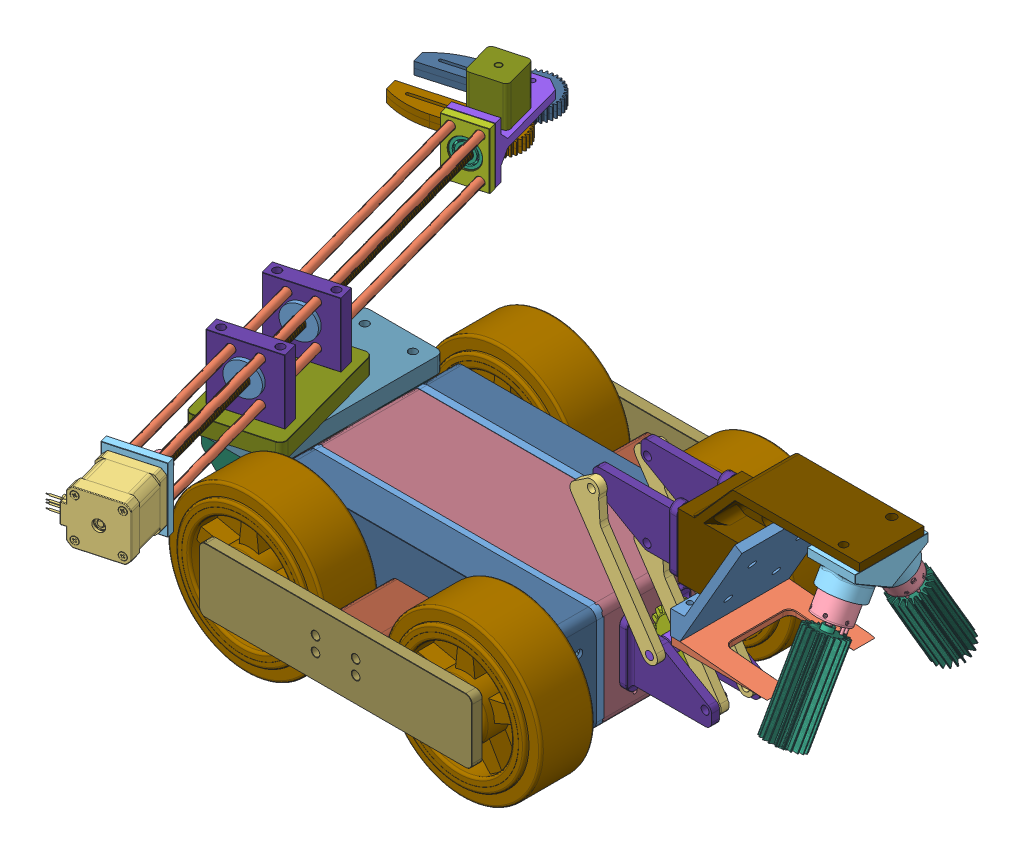
SolidWorks assembly __FINAL_DESIGN, configuration Default. Lengths in mm.
Overall size (608.35 222.7 508.61).
168 component instances, 44 part files, 1 mates.
Components (placement in the parent):
- Chassis-1: Chassis [Default] at origin size (228.6 82.55 202.26)
  - WheelAssy-1: WheelAssy [Default] at origin size (228.6 82.55 139.03)
    - ChassisSidePlate-1: ChassisSidePlate [Default] at origin size (228.6 82.55 6.35)
    - DriveStepper-2: DriveStepper [Default] at (-33.528 0 6.35) x (0 1 0) z (0 0 -1) size (56.9 64.15 97)
    - 60355K503_BALL BEARING-1: 60355K503_BALL BEARING [60355K503] at (85.598 0 1.905) x (-0.923728 -0.383049 0) z (0 0 1) size (15.88 15.88 4.76)
    - 1327K113_MINIATURE 12L14 DRIVE STEEL SHAFT-1: 1327K113_MINIATURE 12L14 DRIVE STEEL SHAFT [1327K113] at (85.598 0 -18.5798) x (-0.959536 -0.281585 0) z (0 0 1) size (6.35 6.35 76.2)
    - 60355K503_BALL BEARING-2: 60355K503_BALL BEARING [60355K503] at (-85.598 0 2.0926) size (15.88 15.88 4.76)
    - 1327K113_MINIATURE 12L14 DRIVE STEEL SHAFT-2: 1327K113_MINIATURE 12L14 DRIVE STEEL SHAFT [1327K113] at (-85.598 0 -16.8162) x (-0.027859 0.999612 0) z (0 0 1) size (6.35 6.35 76.2)
    - 2737T131_FINISHED-BORE SPROCKET FOR ANSI ROLLER CHAIN-1: 2737T131_FINISHED-BORE SPROCKET FOR ANSI ROLLER CHAIN [2737T131] at (85.598 0 -14.478) x (0.999569 0.029358 0) z (0 0 1) size (43.9 43.9 15.88)
    - 2737T131_FINISHED-BORE SPROCKET FOR ANSI ROLLER CHAIN-2: 2737T131_FINISHED-BORE SPROCKET FOR ANSI ROLLER CHAIN [2737T131] at (-85.598 0 -14.478) x (0.999569 0.029358 0) z (0 0 1) size (43.9 43.9 15.88)
    - 6261K281_ROLLER CHAIN-1: 6261K281_ROLLER CHAIN [6261K281] at (-14.2774 -20.8743 -13.97) x (-0.999974 0.007172 0) z (0 0 1) size (18.33 5.99 7.62)
    - 6261K281_ROLLER CHAIN-2: 6261K281_ROLLER CHAIN [6261K281] at (-26.9771 -20.7832 -13.97) x (-0.999974 0.007172 0) z (0 0 1) size (18.33 5.99 7.62)
    - 6261K281_ROLLER CHAIN-3: 6261K281_ROLLER CHAIN [6261K281] at (-39.6768 -20.6921 -13.97) x (-0.999974 0.007172 0) z (0 0 1) size (18.33 5.99 7.62)
    - 6261K281_ROLLER CHAIN-4: 6261K281_ROLLER CHAIN [6261K281] at (-52.3765 -20.601 -13.97) x (-0.999974 0.007172 0) z (0 0 1) size (18.33 5.99 7.62)
    - 6261K281_ROLLER CHAIN-5: 6261K281_ROLLER CHAIN [6261K281] at (-65.0761 -20.5099 -13.97) x (-0.999974 0.007172 0) z (0 0 1) size (18.33 5.99 7.62)
    - 6261K281_ROLLER CHAIN-6: 6261K281_ROLLER CHAIN [6261K281] at (-77.7757 -20.4039 -13.97) x (-0.99993 0.011862 0) z (0 0 1) size (18.33 5.99 7.62)
    - 6261K281_ROLLER CHAIN-7: 6261K281_ROLLER CHAIN [6261K281] at (-90.2233 -19.0521 -13.97) x (-0.92074 0.390177 0) z (0 0 1) size (18.33 5.99 7.62)
    - 6261K281_ROLLER CHAIN-8: 6261K281_ROLLER CHAIN [6261K281] at (-100.614 -12.6055 -13.97) x (-0.510433 0.859918 0) z (0 0 1) size (18.33 5.99 7.62)
    - 6261K281_ROLLER CHAIN-9: 6261K281_ROLLER CHAIN [6261K281] at (-105.1633 -1.2552 -13.97) x (0.098436 0.995143 0) z (0 0 1) size (18.33 5.99 7.62)
    - 6261K281_ROLLER CHAIN-10: 6261K281_ROLLER CHAIN [6261K281] at (-102.1016 10.5834 -13.97) x (0.669012 0.743252 0) z (0 0 1) size (18.33 5.99 7.62)
    - 6261K281_ROLLER CHAIN-11: 6261K281_ROLLER CHAIN [6261K281] at (-92.6199 18.3049 -13.97) x (0.979338 0.20223 0) z (0 0 1) size (18.33 5.99 7.62)
    - 6261K281_ROLLER CHAIN-12: 6261K281_ROLLER CHAIN [6261K281] at (-80.3966 18.9276 -13.97) x (0.911824 -0.41058 0) z (0 0 1) size (18.33 5.99 7.62)
    - 6261K281_ROLLER CHAIN-13: 6261K281_ROLLER CHAIN [6261K281] at (-69.1876 13.0906 -13.97) x (0.794944 -0.606683 0) z (0 0 1) size (18.33 5.99 7.62)
    - 6261K281_ROLLER CHAIN-14: 6261K281_ROLLER CHAIN [6261K281] at (-59.0918 5.3857 -13.97) x (0.794944 -0.606683 0) z (0 0 1) size (18.33 5.99 7.62)
    - 6261K281_ROLLER CHAIN-15: 6261K281_ROLLER CHAIN [6261K281] at (-48.996 -2.3192 -13.97) x (0.794944 -0.606683 0) z (0 0 1) size (18.33 5.99 7.62)
    - 6261K281_ROLLER CHAIN-16: 6261K281_ROLLER CHAIN [6261K281] at (-38.3 -8.6637 -13.97) x (0.983989 -0.178231 0) z (0 0 1) size (18.33 5.99 7.62)
    - 6261K281_ROLLER CHAIN-17: 6261K281_ROLLER CHAIN [6261K281] at (-25.8754 -9.4867 -13.97) x (0.961305 0.275488 0) z (0 0 1) size (18.33 5.99 7.62)
    - 6261K281_ROLLER CHAIN-18: 6261K281_ROLLER CHAIN [6261K281] at (-13.6668 -5.988 -13.97) x (0.961305 0.275488 0) z (0 0 1) size (18.33 5.99 7.62)
    - 6261K281_ROLLER CHAIN-19: 6261K281_ROLLER CHAIN [6261K281] at (-1.4583 -2.4893 -13.97) x (0.961305 0.275488 0) z (0 0 1) size (18.33 5.99 7.62)
    - 6261K281_ROLLER CHAIN-20: 6261K281_ROLLER CHAIN [6261K281] at (10.7503 1.0094 -13.97) x (0.961305 0.275488 0) z (0 0 1) size (18.33 5.99 7.62)
    - 6261K281_ROLLER CHAIN-21: 6261K281_ROLLER CHAIN [6261K281] at (22.9589 4.5081 -13.97) x (0.961305 0.275488 0) z (0 0 1) size (18.33 5.99 7.62)
    - 6261K281_ROLLER CHAIN-22: 6261K281_ROLLER CHAIN [6261K281] at (35.1674 8.0068 -13.97) x (0.961305 0.275488 0) z (0 0 1) size (18.33 5.99 7.62)
    - 6261K281_ROLLER CHAIN-23: 6261K281_ROLLER CHAIN [6261K281] at (47.376 11.5055 -13.97) x (0.961305 0.275488 0) z (0 0 1) size (18.33 5.99 7.62)
    - 6261K281_ROLLER CHAIN-24: 6261K281_ROLLER CHAIN [6261K281] at (59.5846 15.0042 -13.97) x (0.961305 0.275488 0) z (0 0 1) size (18.33 5.99 7.62)
    - 6261K281_ROLLER CHAIN-25: 6261K281_ROLLER CHAIN [6261K281] at (71.796 18.4927 -13.97) x (0.962218 0.272281 0) z (0 0 1) size (18.33 5.99 7.62)
    - 6261K281_ROLLER CHAIN-26: 6261K281_ROLLER CHAIN [6261K281] at (84.1254 20.8259 -13.97) x (0.996634 -0.081984 0) z (0 0 1) size (18.33 5.99 7.62)
    - 6261K281_ROLLER CHAIN-27: 6261K281_ROLLER CHAIN [6261K281] at (96.0889 18.0507 -13.97) x (0.778113 -0.628125 0) z (0 0 1) size (18.33 5.99 7.62)
    - 6261K281_ROLLER CHAIN-28: 6261K281_ROLLER CHAIN [6261K281] at (104.4223 9.0296 -13.97) x (0.290349 -0.956921 0) z (0 0 1) size (18.33 5.99 7.62)
    - 6261K281_ROLLER CHAIN-29: 6261K281_ROLLER CHAIN [6261K281] at (106.2421 -3.116 -13.97) x (-0.297882 -0.954603 0) z (0 0 1) size (18.33 5.99 7.62)
    - 6261K281_ROLLER CHAIN-30: 6261K281_ROLLER CHAIN [6261K281] at (100.9186 -14.1833 -13.97) x (-0.783039 -0.621972 0) z (0 0 1) size (18.33 5.99 7.62)
    - 6261K281_ROLLER CHAIN-31: 6261K281_ROLLER CHAIN [6261K281] at (90.3059 -20.4698 -13.97) x (-0.993471 -0.114084 0) z (0 0 1) size (18.33 5.99 7.62)
    - 6261K281_ROLLER CHAIN-32: 6261K281_ROLLER CHAIN [6261K281] at (77.6681 -21.5337 -13.97) x (-0.999974 0.007172 0) z (0 0 1) size (18.33 5.99 7.62)
    - 6261K281_ROLLER CHAIN-33: 6261K281_ROLLER CHAIN [6261K281] at (64.9685 -21.4426 -13.97) x (-0.999974 0.007172 0) z (0 0 1) size (18.33 5.99 7.62)
    - 6261K281_ROLLER CHAIN-34: 6261K281_ROLLER CHAIN [6261K281] at (52.2688 -21.3515 -13.97) x (-0.999974 0.007172 0) z (0 0 1) size (18.33 5.99 7.62)
    - 6261K281_ROLLER CHAIN-35: 6261K281_ROLLER CHAIN [6261K281] at (39.5691 -21.2604 -13.97) x (-0.999974 0.007172 0) z (0 0 1) size (18.33 5.99 7.62)
    - 6261K281_ROLLER CHAIN-36: 6261K281_ROLLER CHAIN [6261K281] at (26.8695 -21.1694 -13.97) x (-0.999974 0.007172 0) z (0 0 1) size (18.33 5.99 7.62)
    - 6261K281_ROLLER CHAIN-37: 6261K281_ROLLER CHAIN [6261K281] at (14.1698 -21.0783 -13.97) x (-0.999974 0.007172 0) z (0 0 1) size (18.33 5.99 7.62)
    - 6261K281_ROLLER CHAIN-38: 6261K281_ROLLER CHAIN [6261K281] at (1.4701 -20.9872 -13.97) x (-0.999974 0.007172 0) z (0 0 1) size (18.33 5.99 7.62)
    - 6261K281_ROLLER CHAIN-39: 6261K281_ROLLER CHAIN [6261K281] at (-11.2295 -20.8961 -13.97) x (-0.999974 0.007172 0) z (0 0 1) size (18.33 5.99 7.62)
    - 2737T200_FINISHED-BORE SPROCKET FOR ANSI ROLLER CHAIN-3: 2737T200_FINISHED-BORE SPROCKET FOR ANSI ROLLER CHAIN [2737T2] at (-33.528 0 -13.589) x (0.997171 -0.07517 0) z (0 0 1) size (22.55 23.35 12.7)
  - WheelAssy-2: WheelAssy [Default] at (0 0 88.9) x (-1 0 0) z (0 0 -1) size (228.6 82.55 139.03)
    - ChassisSidePlate-1: ChassisSidePlate [Default] at origin size (228.6 82.55 6.35)
    - DriveStepper-2: DriveStepper [Default] at (-33.528 0 6.35) x (0 1 0) z (0 0 -1) size (56.9 64.15 97)
    - 60355K503_BALL BEARING-1: 60355K503_BALL BEARING [60355K503] at (85.598 0 1.905) x (-0.923728 -0.383049 0) z (0 0 1) size (15.88 15.88 4.76)
    - 1327K113_MINIATURE 12L14 DRIVE STEEL SHAFT-1: 1327K113_MINIATURE 12L14 DRIVE STEEL SHAFT [1327K113] at (85.598 0 -18.5798) x (-0.959536 -0.281585 0) z (0 0 1) size (6.35 6.35 76.2)
    - 60355K503_BALL BEARING-2: 60355K503_BALL BEARING [60355K503] at (-85.598 0 2.0926) size (15.88 15.88 4.76)
    - 1327K113_MINIATURE 12L14 DRIVE STEEL SHAFT-2: 1327K113_MINIATURE 12L14 DRIVE STEEL SHAFT [1327K113] at (-85.598 0 -16.8162) x (-0.027859 0.999612 0) z (0 0 1) size (6.35 6.35 76.2)
    - 2737T131_FINISHED-BORE SPROCKET FOR ANSI ROLLER CHAIN-1: 2737T131_FINISHED-BORE SPROCKET FOR ANSI ROLLER CHAIN [2737T131] at (85.598 0 -14.478) x (0.999569 0.029358 0) z (0 0 1) size (43.9 43.9 15.88)
    - 2737T131_FINISHED-BORE SPROCKET FOR ANSI ROLLER CHAIN-2: 2737T131_FINISHED-BORE SPROCKET FOR ANSI ROLLER CHAIN [2737T131] at (-85.598 0 -14.478) x (0.999569 0.029358 0) z (0 0 1) size (43.9 43.9 15.88)
    - 6261K281_ROLLER CHAIN-1: 6261K281_ROLLER CHAIN [6261K281] at (-14.2774 -20.8743 -13.97) x (-0.999974 0.007172 0) z (0 0 1) size (18.33 5.99 7.62)
    - 6261K281_ROLLER CHAIN-2: 6261K281_ROLLER CHAIN [6261K281] at (-26.9771 -20.7832 -13.97) x (-0.999974 0.007172 0) z (0 0 1) size (18.33 5.99 7.62)
    - 6261K281_ROLLER CHAIN-3: 6261K281_ROLLER CHAIN [6261K281] at (-39.6768 -20.6921 -13.97) x (-0.999974 0.007172 0) z (0 0 1) size (18.33 5.99 7.62)
    - 6261K281_ROLLER CHAIN-4: 6261K281_ROLLER CHAIN [6261K281] at (-52.3765 -20.601 -13.97) x (-0.999974 0.007172 0) z (0 0 1) size (18.33 5.99 7.62)
    - 6261K281_ROLLER CHAIN-5: 6261K281_ROLLER CHAIN [6261K281] at (-65.0761 -20.5099 -13.97) x (-0.999974 0.007172 0) z (0 0 1) size (18.33 5.99 7.62)
    - 6261K281_ROLLER CHAIN-6: 6261K281_ROLLER CHAIN [6261K281] at (-77.7757 -20.4039 -13.97) x (-0.99993 0.011862 0) z (0 0 1) size (18.33 5.99 7.62)
    - 6261K281_ROLLER CHAIN-7: 6261K281_ROLLER CHAIN [6261K281] at (-90.2233 -19.0521 -13.97) x (-0.92074 0.390177 0) z (0 0 1) size (18.33 5.99 7.62)
    - 6261K281_ROLLER CHAIN-8: 6261K281_ROLLER CHAIN [6261K281] at (-100.614 -12.6055 -13.97) x (-0.510433 0.859918 0) z (0 0 1) size (18.33 5.99 7.62)
    - 6261K281_ROLLER CHAIN-9: 6261K281_ROLLER CHAIN [6261K281] at (-105.1633 -1.2552 -13.97) x (0.098436 0.995143 0) z (0 0 1) size (18.33 5.99 7.62)
    - 6261K281_ROLLER CHAIN-10: 6261K281_ROLLER CHAIN [6261K281] at (-102.1016 10.5834 -13.97) x (0.669012 0.743252 0) z (0 0 1) size (18.33 5.99 7.62)
    - 6261K281_ROLLER CHAIN-11: 6261K281_ROLLER CHAIN [6261K281] at (-92.6199 18.3049 -13.97) x (0.979338 0.20223 0) z (0 0 1) size (18.33 5.99 7.62)
    - 6261K281_ROLLER CHAIN-12: 6261K281_ROLLER CHAIN [6261K281] at (-80.3966 18.9276 -13.97) x (0.911824 -0.41058 0) z (0 0 1) size (18.33 5.99 7.62)
    - 6261K281_ROLLER CHAIN-13: 6261K281_ROLLER CHAIN [6261K281] at (-69.1876 13.0906 -13.97) x (0.794944 -0.606683 0) z (0 0 1) size (18.33 5.99 7.62)
    - 6261K281_ROLLER CHAIN-14: 6261K281_ROLLER CHAIN [6261K281] at (-59.0918 5.3857 -13.97) x (0.794944 -0.606683 0) z (0 0 1) size (18.33 5.99 7.62)
    - 6261K281_ROLLER CHAIN-15: 6261K281_ROLLER CHAIN [6261K281] at (-48.996 -2.3192 -13.97) x (0.794944 -0.606683 0) z (0 0 1) size (18.33 5.99 7.62)
    - 6261K281_ROLLER CHAIN-16: 6261K281_ROLLER CHAIN [6261K281] at (-38.3 -8.6637 -13.97) x (0.983989 -0.178231 0) z (0 0 1) size (18.33 5.99 7.62)
    - 6261K281_ROLLER CHAIN-17: 6261K281_ROLLER CHAIN [6261K281] at (-25.8754 -9.4867 -13.97) x (0.961305 0.275488 0) z (0 0 1) size (18.33 5.99 7.62)
    - 6261K281_ROLLER CHAIN-18: 6261K281_ROLLER CHAIN [6261K281] at (-13.6668 -5.988 -13.97) x (0.961305 0.275488 0) z (0 0 1) size (18.33 5.99 7.62)
    - 6261K281_ROLLER CHAIN-19: 6261K281_ROLLER CHAIN [6261K281] at (-1.4583 -2.4893 -13.97) x (0.961305 0.275488 0) z (0 0 1) size (18.33 5.99 7.62)
    - 6261K281_ROLLER CHAIN-20: 6261K281_ROLLER CHAIN [6261K281] at (10.7503 1.0094 -13.97) x (0.961305 0.275488 0) z (0 0 1) size (18.33 5.99 7.62)
    - 6261K281_ROLLER CHAIN-21: 6261K281_ROLLER CHAIN [6261K281] at (22.9589 4.5081 -13.97) x (0.961305 0.275488 0) z (0 0 1) size (18.33 5.99 7.62)
    - 6261K281_ROLLER CHAIN-22: 6261K281_ROLLER CHAIN [6261K281] at (35.1674 8.0068 -13.97) x (0.961305 0.275488 0) z (0 0 1) size (18.33 5.99 7.62)
    - 6261K281_ROLLER CHAIN-23: 6261K281_ROLLER CHAIN [6261K281] at (47.376 11.5055 -13.97) x (0.961305 0.275488 0) z (0 0 1) size (18.33 5.99 7.62)
    - 6261K281_ROLLER CHAIN-24: 6261K281_ROLLER CHAIN [6261K281] at (59.5846 15.0042 -13.97) x (0.961305 0.275488 0) z (0 0 1) size (18.33 5.99 7.62)
    - 6261K281_ROLLER CHAIN-25: 6261K281_ROLLER CHAIN [6261K281] at (71.796 18.4927 -13.97) x (0.962218 0.272281 0) z (0 0 1) size (18.33 5.99 7.62)
    - 6261K281_ROLLER CHAIN-26: 6261K281_ROLLER CHAIN [6261K281] at (84.1254 20.8259 -13.97) x (0.996634 -0.081984 0) z (0 0 1) size (18.33 5.99 7.62)
    - 6261K281_ROLLER CHAIN-27: 6261K281_ROLLER CHAIN [6261K281] at (96.0889 18.0507 -13.97) x (0.778113 -0.628125 0) z (0 0 1) size (18.33 5.99 7.62)
    - 6261K281_ROLLER CHAIN-28: 6261K281_ROLLER CHAIN [6261K281] at (104.4223 9.0296 -13.97) x (0.290349 -0.956921 0) z (0 0 1) size (18.33 5.99 7.62)
    - 6261K281_ROLLER CHAIN-29: 6261K281_ROLLER CHAIN [6261K281] at (106.2421 -3.116 -13.97) x (-0.297882 -0.954603 0) z (0 0 1) size (18.33 5.99 7.62)
    - 6261K281_ROLLER CHAIN-30: 6261K281_ROLLER CHAIN [6261K281] at (100.9186 -14.1833 -13.97) x (-0.783039 -0.621972 0) z (0 0 1) size (18.33 5.99 7.62)
    - 6261K281_ROLLER CHAIN-31: 6261K281_ROLLER CHAIN [6261K281] at (90.3059 -20.4698 -13.97) x (-0.993471 -0.114084 0) z (0 0 1) size (18.33 5.99 7.62)
    - 6261K281_ROLLER CHAIN-32: 6261K281_ROLLER CHAIN [6261K281] at (77.6681 -21.5337 -13.97) x (-0.999974 0.007172 0) z (0 0 1) size (18.33 5.99 7.62)
    - 6261K281_ROLLER CHAIN-33: 6261K281_ROLLER CHAIN [6261K281] at (64.9685 -21.4426 -13.97) x (-0.999974 0.007172 0) z (0 0 1) size (18.33 5.99 7.62)
    - 6261K281_ROLLER CHAIN-34: 6261K281_ROLLER CHAIN [6261K281] at (52.2688 -21.3515 -13.97) x (-0.999974 0.007172 0) z (0 0 1) size (18.33 5.99 7.62)
    - 6261K281_ROLLER CHAIN-35: 6261K281_ROLLER CHAIN [6261K281] at (39.5691 -21.2604 -13.97) x (-0.999974 0.007172 0) z (0 0 1) size (18.33 5.99 7.62)
    - 6261K281_ROLLER CHAIN-36: 6261K281_ROLLER CHAIN [6261K281] at (26.8695 -21.1694 -13.97) x (-0.999974 0.007172 0) z (0 0 1) size (18.33 5.99 7.62)
    - 6261K281_ROLLER CHAIN-37: 6261K281_ROLLER CHAIN [6261K281] at (14.1698 -21.0783 -13.97) x (-0.999974 0.007172 0) z (0 0 1) size (18.33 5.99 7.62)
    - 6261K281_ROLLER CHAIN-38: 6261K281_ROLLER CHAIN [6261K281] at (1.4701 -20.9872 -13.97) x (-0.999974 0.007172 0) z (0 0 1) size (18.33 5.99 7.62)
    - 6261K281_ROLLER CHAIN-39: 6261K281_ROLLER CHAIN [6261K281] at (-11.2295 -20.8961 -13.97) x (-0.999974 0.007172 0) z (0 0 1) size (18.33 5.99 7.62)
    - 2737T200_FINISHED-BORE SPROCKET FOR ANSI ROLLER CHAIN-3: 2737T200_FINISHED-BORE SPROCKET FOR ANSI ROLLER CHAIN [2737T2] at (-33.528 0 -13.589) x (0.997171 -0.07517 0) z (0 0 1) size (22.55 23.35 12.7)
- Wheels-1: Wheels [Default] at origin size (295.66 124.46 255.27)
  - Wheel_Bushing-1: Wheel_Bushing [Default] at (85.598 0 -83.185) x (0.988756 0.149539 0) z (0 0 1) size (28.7 28.7 54.61)
  - Wheel_Bushing-2: Wheel_Bushing [Default] at (-85.598 0 -83.185) x (0.931602 -0.363481 0) z (0 0 1) size (28.7 28.7 54.61)
  - Wheel_Bushing-3: Wheel_Bushing [Default] at (85.598 0 117.475) x (0.988134 -0.153594 0) z (0 0 1) size (28.7 28.7 54.61)
  - Wheel_Bushing-4: Wheel_Bushing [Default] at (-85.598 0 117.475) x (0.990561 0.137069 0) z (0 0 1) size (28.7 28.7 54.61)
  - CasterWheel_5in.ipt-1: CasterWheel_5in.ipt [Default] at (-85.598 0 144.78) size (124.46 124.46 54.61)
  - CasterWheel_5in.ipt-2: CasterWheel_5in.ipt [Default] at (85.598 0 144.78) size (124.46 124.46 54.61)
  - CasterWheel_5in.ipt-3: CasterWheel_5in.ipt [Default] at (-85.598 0 -55.88) size (124.46 124.46 54.61)
  - CasterWheel_5in.ipt-4: CasterWheel_5in.ipt [Default] at (85.598 0 -55.88) size (124.46 124.46 54.61)
- ChassisAcc-1: ChassisAcc [Default] at origin size (228.6 82.55 272.8)
  - ChassisSideCover-1: ChassisSideCover [Default] at (0 0 -27.686) size (228.6 82.55 27.94)
  - ChassisSideCover-2: ChassisSideCover [Default] at (0 0 116.586) x (1 0 0) z (0 0 -1) size (228.6 82.55 27.94)
  - SideSensorEntension-1: SideSensorEntension [Default] at (0 -0.0176 -83.566) size (40.64 25.4 55.88)
  - SideSensorEntension-2: SideSensorEntension [Default] at (0 -0.0176 116.586) size (40.64 25.4 55.88)
  - SideSensorMount-1: SideSensorMount [Default] at (0 -0.0176 172.466) size (215.9 50.8 8.38)
  - SideSensorMount-2: SideSensorMount [Default] at (0 -0.0176 -91.948) size (215.9 50.8 8.38)
- ChassisMotorHousing-3: ChassisMotorHousing [Default] at (0 0 6.35) size (228.6 82.55 77.47)
- CubeClawAssy-1: CubeClawAssy [Default] at origin size (227.38 147.32 508.61)
  - ClawArmBearingMount-1: ClawArmBearingMount [Default] at (-152.4 31.877 44.45) x (0 0 1) z (-1 0 0) size (139.7 12.7 63.5)
  - 60355K509_BALL BEARING-1: 60355K509_BALL BEARING [60355K509] at (-152.4 36.6395 73.406) x (-0.297226 0 -0.954807) z (0 1 0) size (50.8 50.8 9.53)
  - ArmRotate-1: ArmRotate [Default] at (-152.4 57.277 73.406) x (0.265648 0 0.96407) z (0.96407 0 -0.265648) size (101.6 63.5 63.5)
  - RackStand-1: RackStand [Default] at (-160.8343 57.277 42.7968) x (0.265648 0 0.96407) z (-0.96407 0 0.265648) size (12 50.8 50.8)
  - RackStand-2: RackStand [Default] at (-143.9657 57.277 104.0152) x (0.265648 0 0.96407) z (-0.96407 0 0.265648) size (12 50.8 50.8)
  - 93410A912_ASTM A193 STEEL ACME LEAD SCREW-1: 93410A912_ASTM A193 STEEL ACME LEAD SCREW [93410A912] at (-159.5487 84.582 47.4626) x (0.957787 0.113984 -0.263917) z (-0.265648 0 -0.96407) size (11 9.53 384.84)
  - 95120A592_BRONZE GENERAL PURPOSE ACME FLANGE NUT-1: 95120A592_BRONZE GENERAL PURPOSE ACME FLANGE NUT [95120A592] at (-158.3968 84.582 51.643) x (0.935858 -0.240148 -0.257875) z (0.231519 0.970736 -0.063795) size (25.4 22.84 25.4)
  - 95120A592_BRONZE GENERAL PURPOSE ACME FLANGE NUT-2: 95120A592_BRONZE GENERAL PURPOSE ACME FLANGE NUT [95120A592] at (-141.5281 84.582 112.8615) x (0.890426 -0.383331 -0.245356) z (0.369558 0.923611 -0.101831) size (25.4 22.84 25.4)
  - Rail-1: Rail [Default] at (-200.9719 68.707 -138.723) x (0.963827 0.022472 -0.265581) z (0.265648 0 0.96407) size (6.35 6.35 381)
  - Rail-2: Rail [Default] at (-219.3375 68.707 -133.6624) x (0.963827 0.022472 -0.265581) z (0.265648 0 0.96407) size (6.35 6.35 381)
  - Rail-3: Rail [Default] at (-219.3375 100.457 -133.6624) x (-0.624115 0.762171 0.171974) z (0.265648 0 0.96407) size (6.35 6.35 381)
  - Rail-4: Rail [Default] at (-200.9719 100.457 -138.723) x (0.963827 0.022472 -0.265581) z (0.265648 0 0.96407) size (6.35 6.35 381)
  - nema_17_motor-1: nema_17_motor [Varsayılan] at (-108.9426 84.582 231.1179) x (0 -1 0) z (-0.265648 0 -0.96407) size (42 58.5 65.65)
  - ClawWormCoupler-1: ClawWormCoupler [Default] at (-117.5497 84.582 199.8821) x (0.587821 0.792611 -0.161973) z (0.265648 0 0.96407) size (13.97 13.97 25.4)
  - ClawRailMotorBracket-1: ClawRailMotorBracket [Default] at (-110.6295 84.582 224.9961) x (0.96407 0 -0.265648) z (0.265648 0 0.96407) size (43.18 50.8 6.35)
  - 60355K504_BALL BEARING-1: 60355K504_BALL BEARING [60355K504] at (-209.4167 84.582 -133.5144) x (-0.963827 -0.022472 0.265581) z (0.265648 0 0.96407) size (22.23 22.23 5.56)
  - ClawBracket-1: ClawBracket [Default] at (-210.1547 84.582 -136.1927) x (0.96407 0 -0.265648) z (0.265648 0 0.96407) size (31.75 44.45 6.35)
  - ClawMount-1: ClawMount [Default] at (-194.8501 62.357 -140.4099) x (-0.96407 0 0.265648) z (-0.265648 0 -0.96407) size (31.75 44.45 76.2)
  - CLAW_L-1: CLAW_L [Default] at (-218.589 76.6445 -166.8019) x (-0.262286 0 -0.96499) z (0 -1 0) size (40.21 91.53 4.76)
  - CLAW_L-2: CLAW_L [Default] at (-218.589 81.407 -166.8019) x (-0.262286 0 -0.96499) z (0 -1 0) size (40.21 91.53 4.76)
  - CLAW_R-1: CLAW_R [Default] at (-228.7102 76.6445 -203.533) x (-0.274481 0 -0.961592) z (0 -1 0) size (40.15 91.5 4.76)
  - CLAW_R-2: CLAW_R [Default] at (-228.7102 81.407 -203.533) x (-0.274481 0 -0.961592) z (0 -1 0) size (40.15 91.5 4.76)
  - 57545K511_SPEED-REDUCING WORM GEAR FOR 90 DEG TRANSFER-1: 57545K511_SPEED-REDUCING WORM GEAR FOR 90 DEG TRANSFER [57545K511] at (-152.4 0.127 73.406) x (-0.122179 0 0.992508) z (-0.992508 0 -0.122179) size (44.78 28.61 44.18)
  - 57545K527_SPEED-REDUCING WORM GEAR FOR 90 DEG TRANSFER-2: 57545K527_SPEED-REDUCING WORM GEAR FOR 90 DEG TRANSFER [57545K527] at (-151.281 0.382 40.4015) x (0 0.509771 -0.86031) z (1 0 0) size (31.13 29.72 30.93)
  - RotationBushing-1: RotationBushing [Default] at (-111.5935 0.382 40.4015) x (0 -0.164114 0.986441) z (-1 0 0) size (12.7 12.7 53.98)
  - 6627T380_POSITION-CONTROL DC MOTOR-1: 6627T380_POSITION-CONTROL DC MOTOR [6627T38] at (-109.5615 0.382 40.4015) x (0 0 1) z (-1 0 0) size (35.31 35.31 49.28)
  - CubeArmMountBracket-3: CubeArmMountBracket [Default] at (-127 25.527 -7.3307) x (0 -1 0) z (0 0 -1) size (57.15 63.5 12.7)
  - CubeArmMountBracket-4: CubeArmMountBracket [Default] at (-127 25.273 109.0013) x (0 -1 0) z (0 0 -1) size (57.15 63.5 12.7)
  - 6627T370_POSITION-CONTROL DC MOTOR-1: 6627T370_POSITION-CONTROL DC MOTOR [6627T37] at (-218.589 89.789 -166.8019) x (0.96407 0 -0.265648) z (0 -1 0) size (28.19 28.19 52.07)
- LiftAssy-1: LiftAssy [Default] at origin size (229.52 194.08 170.22)
  - LiftLinkageBaseMount-1: LiftLinkageBaseMount [Default] at (120.65 -15.875 60.96) size (69.85 50.85 12.75)
  - LiftLinkageBaseMount-2: LiftLinkageBaseMount [Default] at (120.65 -15.875 22.86) size (69.85 50.85 12.75)
  - LiftLinkageBaseMount-3: LiftLinkageBaseMount [Default] at (153.714 119.8304 60.96) x (-1 0 0) z (0 0 1) size (69.85 50.85 12.75)
  - LiftLinkageBaseMount-4: LiftLinkageBaseMount [Default] at (153.714 119.8304 22.86) x (-1 0 0) z (0 0 1) size (69.85 50.85 12.75)
  - PyrIntakeAngledMount-1: PyrIntakeAngledMount [Default] at (185.464 100.7804 70.485) x (-1 0 0) z (0 0 -1) size (144.52 85.09 50.8)
  - PyrIntakeBacking-1: PyrIntakeBacking [Default] at (198.164 97.3774 45.085) x (0 0 -1) z (0.866025 -0.5 0) size (86.36 101.6 15.88)
  - PyrIntakeForks-1: PyrIntakeForks [Default] at (210.9742 47.0333 45.085) x (0 0 -1) z (0 1 0) size (86.36 75.73 6.35)
  - LiftLinkage-6: LiftLinkage [Default] at (141.2859 17.145 22.86) x (-0.830828 -0.556529 0) z (0 0 -1) size (25.4 114.3 6.35)
  - LiftLinkage-7: LiftLinkage [Default] at (141.2859 17.145 73.66) x (-0.830828 -0.556529 0) z (0 0 -1) size (25.4 114.3 6.35)
  - LiftLinkage-8: LiftLinkage [Default] at (179.07 -4.6697 35.56) x (-0.830828 -0.556529 0) z (0 0 -1) size (25.4 114.3 6.35)
  - LiftLinkage-9: LiftLinkage [Default] at (179.07 -4.6697 60.96) x (-0.830828 -0.556529 0) z (0 0 -1) size (25.4 114.3 6.35)
  - PyrIntakeFlapperMotor-3: PyrIntakeFlapperMotor [Default] at (285.5319 139.3925 59.596) x (0 -0.866025 0.5) z (0.343501 0.469576 0.81333) size (45.7 26.82 26.82)
  - PyrIntakeFlapperMotor-4: PyrIntakeFlapperMotor [Default] at (285.5319 139.3925 30.574) x (0 -0.866025 -0.5) z (-0.923977 -0.191224 0.331209) size (45.7 26.82 26.82)
  - PyrIntakeMotorMount-1: PyrIntakeMotorMount [Default] at (304.5819 131.0146 45.085) x (0 0 1) z (-1 0 0) size (70.32 33.98 38.1)
  - PyrIntakeRoller-1: PyrIntakeRoller [Default] at (285.5319 78.8205 -4.3972) x (0.918298 -0.197945 0.342851) z (-0.39589 -0.459149 0.795269) size (30.23 75 30.45)
  - PyrIntakeRoller-2: PyrIntakeRoller [Default] at (285.5319 78.8205 94.5672) x (0.955222 0.147946 0.256249) z (-0.295891 0.477611 0.827246) size (30.23 75 30.45)
  - 57545K527_SPEED-REDUCING WORM GEAR FOR 90 DEG TRANSFER-1: 57545K527_SPEED-REDUCING WORM GEAR FOR 90 DEG TRANSFER [57545K527] at (140.5014 -15.9576 44.6236) x (0 0.051502 -0.998673) z (1 0 0) size (31.13 29.72 30.93)
  - 57545K511_SPEED-REDUCING WORM GEAR FOR 90 DEG TRANSFER-cutoff-1: 57545K511_SPEED-REDUCING WORM GEAR FOR 90 DEG TRANSFER-cutoff [57545K511] at (141.2859 17.145 45.4541) x (0.997471 0.071068 0) z (0.071068 -0.997471 0) size (44.78 13.14 44.18)
  - RotationBushing-1: RotationBushing [Default] at (113.811 -15.9576 44.6236) x (0 0 -1) z (1 0 0) size (12.7 12.7 53.98)
  - 6627T380_POSITION-CONTROL DC MOTOR-1: 6627T380_POSITION-CONTROL DC MOTOR [6627T38] at (111.779 -15.9576 44.6236) x (0 0 -1) z (1 0 0) size (35.31 35.31 49.28)
  - PyrIntakeLinkageRod-1: PyrIntakeLinkageRod [Default] at (141.2859 17.145 16.51) size (12.7 12.7 57.15)
Mates (geometry in assembly coordinates):
- Coincident1: coincident anti-aligned: plane of Chassis-1/WheelAssy-1/ChassisSidePlate-1 through (0 0 6.35) normal (0 0 1); plane of ChassisMotorHousing-3 through (107.95 34.925 6.35) normal (0 0 -1)
